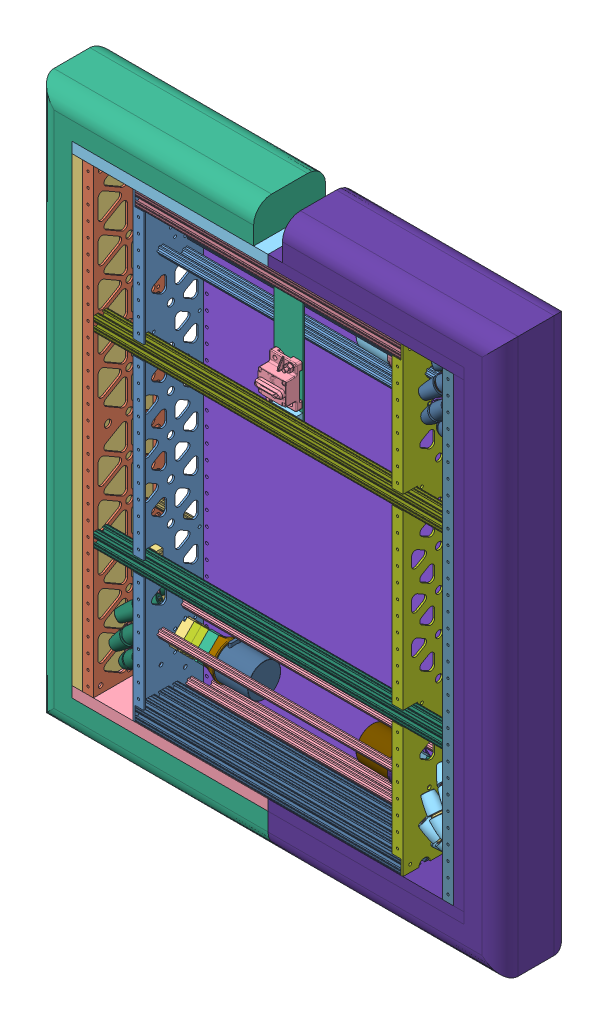
SolidWorks assembly Copy of Fame 2020, configuration Default. Lengths in mm. (continued)
Components (placement in the parent): (continued)
- Left Wheel Assembly v4(Mirror) (2)^Copy of Fame 2020-1: Left Wheel Assembly v4(Mirror) (2)^Copy of Fame 2020 [Default] at (500 0 0) x (1 0 0) z (0 0 -1) size (65.82 166.11 165.01) (virtual)
  - 6_Mecanum_Wheel_Left_217-2799 v1(Mirror) (2)^Left Wheel Assembly v4(Mirror) (2)_Copy of Fame 2020-1: 6_Mecanum_Wheel_Left_217-2799 v1(Mirror) (2)^Left Wheel Assembly v4(Mirror) (2)_Copy of Fame 2020 [Default] x (0 0 -1) z (1 0 0) size (165.01 166.11 65.82) (virtual)
    - 217-2799-001 Rev1(Mirror) (2)^6_Mecanum_Wheel_Left_217-2799 v1(Mirror) (2)_Left Wheel Assembly v4(Mirror) (2)_Copy of Fame 2020-1: 217-2799-001 Rev1(Mirror) (2)^6_Mecanum_Wheel_Left_217-2799 v1(Mirror) (2)_Left Wheel Assembly v4(Mirror) (2)_Copy of Fame 2020 [Default] at (33.3875 -317.5 -234.0098) x (0.707107 0.707107 0) z (0 0 1) size (95.78 100.46 28.55) (virtual)
    - 217-2799-001 Rev1(Mirror) (2)^6_Mecanum_Wheel_Left_217-2799 v1(Mirror) (2)_Left Wheel Assembly v4(Mirror) (2)_Copy of Fame 2020-2: 217-2799-001 Rev1(Mirror) (2)^6_Mecanum_Wheel_Left_217-2799 v1(Mirror) (2)_Left Wheel Assembly v4(Mirror) (2)_Copy of Fame 2020 [Default] at (33.3875 -317.5 -221.3098) x (-0.987688 -0.156434 0) z (0 0 -1) size (95.78 100.46 28.55) (virtual)
    - 217-2799-002 Rev1(Mirror) (2)^6_Mecanum_Wheel_Left_217-2799 v1(Mirror) (2)_Left Wheel Assembly v4(Mirror) (2)_Copy of Fame 2020-1: 217-2799-002 Rev1(Mirror) (2)^6_Mecanum_Wheel_Left_217-2799 v1(Mirror) (2)_Left Wheel Assembly v4(Mirror) (2)_Copy of Fame 2020 [Default] at (4.057 -346.8305 -227.6598) x (-0.707107 0.707107 0) z (0.707107 0.707107 0) size (26.84 25.39 30.1) (virtual)
    - 217-2799-002 Rev1(Mirror) (2)^6_Mecanum_Wheel_Left_217-2799 v1(Mirror) (2)_Left Wheel Assembly v4(Mirror) (2)_Copy of Fame 2020-2: 217-2799-002 Rev1(Mirror) (2)^6_Mecanum_Wheel_Left_217-2799 v1(Mirror) (2)_Left Wheel Assembly v4(Mirror) (2)_Copy of Fame 2020 [Default] at (-7.5815 -323.9888 -227.6598) x (-0.156434 0.987688 0) z (0.987688 0.156434 0) size (26.84 25.39 30.1) (virtual)
    - 217-2799-002 Rev1(Mirror) (2)^6_Mecanum_Wheel_Left_217-2799 v1(Mirror) (2)_Left Wheel Assembly v4(Mirror) (2)_Copy of Fame 2020-3: 217-2799-002 Rev1(Mirror) (2)^6_Mecanum_Wheel_Left_217-2799 v1(Mirror) (2)_Left Wheel Assembly v4(Mirror) (2)_Copy of Fame 2020 [Default] at (-3.5711 -298.6686 -227.6598) x (0.45399 0.891007 0) z (0.891007 -0.45399 0) size (26.84 25.39 30.1) (virtual)
    - 217-2799-002 Rev1(Mirror) (2)^6_Mecanum_Wheel_Left_217-2799 v1(Mirror) (2)_Left Wheel Assembly v4(Mirror) (2)_Copy of Fame 2020-4: 217-2799-002 Rev1(Mirror) (2)^6_Mecanum_Wheel_Left_217-2799 v1(Mirror) (2)_Left Wheel Assembly v4(Mirror) (2)_Copy of Fame 2020 [Default] at (14.5561 -280.5414 -227.6598) x (0.891007 0.45399 0) z (0.45399 -0.891007 0) size (26.84 25.39 30.1) (virtual)
    - 217-2799-002 Rev1(Mirror) (2)^6_Mecanum_Wheel_Left_217-2799 v1(Mirror) (2)_Left Wheel Assembly v4(Mirror) (2)_Copy of Fame 2020-5: 217-2799-002 Rev1(Mirror) (2)^6_Mecanum_Wheel_Left_217-2799 v1(Mirror) (2)_Left Wheel Assembly v4(Mirror) (2)_Copy of Fame 2020 [Default] at (39.8763 -276.531 -227.6598) x (0.987688 -0.156434 0) z (-0.156434 -0.987688 0) size (26.84 25.39 30.1) (virtual)
    - 217-2799-002 Rev1(Mirror) (2)^6_Mecanum_Wheel_Left_217-2799 v1(Mirror) (2)_Left Wheel Assembly v4(Mirror) (2)_Copy of Fame 2020-6: 217-2799-002 Rev1(Mirror) (2)^6_Mecanum_Wheel_Left_217-2799 v1(Mirror) (2)_Left Wheel Assembly v4(Mirror) (2)_Copy of Fame 2020 [Default] at (62.718 -288.1695 -227.6598) x (0.707107 -0.707107 0) z (-0.707107 -0.707107 0) size (26.84 25.39 30.1) (virtual)
    - 217-2799-002 Rev1(Mirror) (2)^6_Mecanum_Wheel_Left_217-2799 v1(Mirror) (2)_Left Wheel Assembly v4(Mirror) (2)_Copy of Fame 2020-7: 217-2799-002 Rev1(Mirror) (2)^6_Mecanum_Wheel_Left_217-2799 v1(Mirror) (2)_Left Wheel Assembly v4(Mirror) (2)_Copy of Fame 2020 [Default] at (74.3565 -311.0112 -227.6598) x (0.156434 -0.987688 0) z (-0.987688 -0.156434 0) size (26.84 25.39 30.1) (virtual)
    - 217-2799-002 Rev1(Mirror) (2)^6_Mecanum_Wheel_Left_217-2799 v1(Mirror) (2)_Left Wheel Assembly v4(Mirror) (2)_Copy of Fame 2020-8: 217-2799-002 Rev1(Mirror) (2)^6_Mecanum_Wheel_Left_217-2799 v1(Mirror) (2)_Left Wheel Assembly v4(Mirror) (2)_Copy of Fame 2020 [Default] at (70.3461 -336.3314 -227.6598) x (-0.45399 -0.891007 0) z (-0.891007 0.45399 0) size (26.84 25.39 30.1) (virtual)
    - 217-2799-002 Rev1(Mirror) (2)^6_Mecanum_Wheel_Left_217-2799 v1(Mirror) (2)_Left Wheel Assembly v4(Mirror) (2)_Copy of Fame 2020-9: 217-2799-002 Rev1(Mirror) (2)^6_Mecanum_Wheel_Left_217-2799 v1(Mirror) (2)_Left Wheel Assembly v4(Mirror) (2)_Copy of Fame 2020 [Default] at (52.2189 -354.4586 -227.6598) x (-0.891007 -0.45399 0) z (-0.45399 0.891007 0) size (26.84 25.39 30.1) (virtual)
    - 217-2799-002 Rev1(Mirror) (2)^6_Mecanum_Wheel_Left_217-2799 v1(Mirror) (2)_Left Wheel Assembly v4(Mirror) (2)_Copy of Fame 2020-10: 217-2799-002 Rev1(Mirror) (2)^6_Mecanum_Wheel_Left_217-2799 v1(Mirror) (2)_Left Wheel Assembly v4(Mirror) (2)_Copy of Fame 2020 [Default] at (26.8987 -358.469 -227.6598) x (-0.987688 0.156434 0) z (0.156434 0.987688 0) size (26.84 25.39 30.1) (virtual)
    - 217-2586-003 Rev2(Mirror) (2)^6_Mecanum_Wheel_Left_217-2799 v1(Mirror) (2)_Left Wheel Assembly v4(Mirror) (2)_Copy of Fame 2020-1: 217-2586-003 Rev2(Mirror) (2)^6_Mecanum_Wheel_Left_217-2799 v1(Mirror) (2)_Left Wheel Assembly v4(Mirror) (2)_Copy of Fame 2020 [Default] at (-13.4676 -358.6894 -223.6536) x (0.41944 0.854155 -0.30739) z (0.757674 -0.142894 0.636798) size (19.46 28.57 19.46) (virtual)
    - 217-2586-003 Rev2(Mirror) (2)^6_Mecanum_Wheel_Left_217-2799 v1(Mirror) (2)_Left Wheel Assembly v4(Mirror) (2)_Copy of Fame 2020-2: 217-2586-003 Rev2(Mirror) (2)^6_Mecanum_Wheel_Left_217-2799 v1(Mirror) (2)_Left Wheel Assembly v4(Mirror) (2)_Copy of Fame 2020 [Default] at (-7.8019 -364.3551 -231.666) x (0.847342 0.451134 0.280161) z (-0.17892 0.739241 -0.649238) size (19.46 28.57 19.46) (virtual)
    - 217-2586-003 Rev2(Mirror) (2)^6_Mecanum_Wheel_Left_217-2799 v1(Mirror) (2)_Left Wheel Assembly v4(Mirror) (2)_Copy of Fame 2020-3: 217-2586-003 Rev2(Mirror) (2)^6_Mecanum_Wheel_Left_217-2799 v1(Mirror) (2)_Left Wheel Assembly v4(Mirror) (2)_Copy of Fame 2020 [Default] at (-27.4761 -331.196 -231.666) x (0.950684 -0.13308 0.280161) z (0.289766 0.703225 -0.649238) size (19.46 28.57 19.46) (virtual)
    - 217-2586-003 Rev2(Mirror) (2)^6_Mecanum_Wheel_Left_217-2799 v1(Mirror) (2)_Left Wheel Assembly v4(Mirror) (2)_Copy of Fame 2020-4: 217-2586-003 Rev2(Mirror) (2)^6_Mecanum_Wheel_Left_217-2799 v1(Mirror) (2)_Left Wheel Assembly v4(Mirror) (2)_Copy of Fame 2020 [Default] at (-23.9025 -292.8056 -231.666) x (0.690897 -0.666462 0.280161) z (0.647771 0.398601 -0.649238) size (19.46 28.57 19.46) (virtual)
    - 217-2586-003 Rev2(Mirror) (2)^6_Mecanum_Wheel_Left_217-2799 v1(Mirror) (2)_Left Wheel Assembly v4(Mirror) (2)_Copy of Fame 2020-5: 217-2586-003 Rev2(Mirror) (2)^6_Mecanum_Wheel_Left_217-2799 v1(Mirror) (2)_Left Wheel Assembly v4(Mirror) (2)_Copy of Fame 2020 [Default] at (1.5539 -263.8475 -231.666) x (0.167211 -0.945278 0.280161) z (0.75835 -0.058276 -0.649238) size (19.46 28.57 19.46) (virtual)
    - 217-2586-003 Rev2(Mirror) (2)^6_Mecanum_Wheel_Left_217-2799 v1(Mirror) (2)_Left Wheel Assembly v4(Mirror) (2)_Copy of Fame 2020-6: 217-2586-003 Rev2(Mirror) (2)^6_Mecanum_Wheel_Left_217-2799 v1(Mirror) (2)_Left Wheel Assembly v4(Mirror) (2)_Copy of Fame 2020 [Default] at (39.1697 -255.3829 -231.666) x (-0.420344 -0.86303 0.280161) z (0.579264 -0.492893 -0.649238) size (19.46 28.57 19.46) (virtual)
    - 217-2586-003 Rev2(Mirror) (2)^6_Mecanum_Wheel_Left_217-2799 v1(Mirror) (2)_Left Wheel Assembly v4(Mirror) (2)_Copy of Fame 2020-7: 217-2586-003 Rev2(Mirror) (2)^6_Mecanum_Wheel_Left_217-2799 v1(Mirror) (2)_Left Wheel Assembly v4(Mirror) (2)_Copy of Fame 2020 [Default] at (74.5769 -270.6449 -231.666) x (-0.847342 -0.451134 0.280161) z (0.17892 -0.739241 -0.649238) size (19.46 28.57 19.46) (virtual)
    - 217-2586-003 Rev2(Mirror) (2)^6_Mecanum_Wheel_Left_217-2799 v1(Mirror) (2)_Left Wheel Assembly v4(Mirror) (2)_Copy of Fame 2020-8: 217-2586-003 Rev2(Mirror) (2)^6_Mecanum_Wheel_Left_217-2799 v1(Mirror) (2)_Left Wheel Assembly v4(Mirror) (2)_Copy of Fame 2020 [Default] at (94.2511 -303.804 -231.666) x (-0.950684 0.13308 0.280161) z (-0.289766 -0.703225 -0.649238) size (19.46 28.57 19.46) (virtual)
    - 217-2586-003 Rev2(Mirror) (2)^6_Mecanum_Wheel_Left_217-2799 v1(Mirror) (2)_Left Wheel Assembly v4(Mirror) (2)_Copy of Fame 2020-9: 217-2586-003 Rev2(Mirror) (2)^6_Mecanum_Wheel_Left_217-2799 v1(Mirror) (2)_Left Wheel Assembly v4(Mirror) (2)_Copy of Fame 2020 [Default] at (90.6775 -342.1944 -231.666) x (-0.690897 0.666462 0.280161) z (-0.647771 -0.398601 -0.649238) size (19.46 28.57 19.46) (virtual)
    - 217-2586-003 Rev2(Mirror) (2)^6_Mecanum_Wheel_Left_217-2799 v1(Mirror) (2)_Left Wheel Assembly v4(Mirror) (2)_Copy of Fame 2020-10: 217-2586-003 Rev2(Mirror) (2)^6_Mecanum_Wheel_Left_217-2799 v1(Mirror) (2)_Left Wheel Assembly v4(Mirror) (2)_Copy of Fame 2020 [Default] at (65.2211 -371.1525 -231.666) x (-0.167211 0.945278 0.280161) z (-0.75835 0.058276 -0.649238) size (19.46 28.57 19.46) (virtual)
    - 217-2586-003 Rev2(Mirror) (2)^6_Mecanum_Wheel_Left_217-2799 v1(Mirror) (2)_Left Wheel Assembly v4(Mirror) (2)_Copy of Fame 2020-11: 217-2586-003 Rev2(Mirror) (2)^6_Mecanum_Wheel_Left_217-2799 v1(Mirror) (2)_Left Wheel Assembly v4(Mirror) (2)_Copy of Fame 2020 [Default] at (27.6053 -379.6171 -231.666) x (0.420344 0.86303 0.280161) z (-0.579264 0.492893 -0.649238) size (19.46 28.57 19.46) (virtual)
    - 217-2586-003 Rev2(Mirror) (2)^6_Mecanum_Wheel_Left_217-2799 v1(Mirror) (2)_Left Wheel Assembly v4(Mirror) (2)_Copy of Fame 2020-12: 217-2586-003 Rev2(Mirror) (2)^6_Mecanum_Wheel_Left_217-2799 v1(Mirror) (2)_Left Wheel Assembly v4(Mirror) (2)_Copy of Fame 2020 [Default] at (-28.7296 -323.2822 -223.6536) x (0.841394 0.444485 -0.30739) z (0.52898 -0.560953 0.636798) size (19.46 28.57 19.46) (virtual)
    - 217-2586-003 Rev2(Mirror) (2)^6_Mecanum_Wheel_Left_217-2799 v1(Mirror) (2)_Left Wheel Assembly v4(Mirror) (2)_Copy of Fame 2020-13: 217-2586-003 Rev2(Mirror) (2)^6_Mecanum_Wheel_Left_217-2799 v1(Mirror) (2)_Left Wheel Assembly v4(Mirror) (2)_Copy of Fame 2020 [Default] at (-20.265 -285.6664 -223.6536) x (0.941964 -0.134963 -0.30739) z (0.098234 -0.764747 0.636798) size (19.46 28.57 19.46) (virtual)
    - 217-2586-003 Rev2(Mirror) (2)^6_Mecanum_Wheel_Left_217-2799 v1(Mirror) (2)_Left Wheel Assembly v4(Mirror) (2)_Copy of Fame 2020-14: 217-2586-003 Rev2(Mirror) (2)^6_Mecanum_Wheel_Left_217-2799 v1(Mirror) (2)_Left Wheel Assembly v4(Mirror) (2)_Copy of Fame 2020 [Default] at (8.6931 -260.21 -223.6536) x (0.682736 -0.66286 -0.30739) z (-0.370035 -0.676434 0.636798) size (19.46 28.57 19.46) (virtual)
    - 217-2586-003 Rev2(Mirror) (2)^6_Mecanum_Wheel_Left_217-2799 v1(Mirror) (2)_Left Wheel Assembly v4(Mirror) (2)_Copy of Fame 2020-15: 217-2586-003 Rev2(Mirror) (2)^6_Mecanum_Wheel_Left_217-2799 v1(Mirror) (2)_Left Wheel Assembly v4(Mirror) (2)_Copy of Fame 2020 [Default] at (47.0835 -256.6364 -223.6536) x (0.162726 -0.937567 -0.30739) z (-0.696962 -0.329746 0.636798) size (19.46 28.57 19.46) (virtual)
    - 217-2586-003 Rev2(Mirror) (2)^6_Mecanum_Wheel_Left_217-2799 v1(Mirror) (2)_Left Wheel Assembly v4(Mirror) (2)_Copy of Fame 2020-16: 217-2586-003 Rev2(Mirror) (2)^6_Mecanum_Wheel_Left_217-2799 v1(Mirror) (2)_Left Wheel Assembly v4(Mirror) (2)_Copy of Fame 2020 [Default] at (80.2426 -276.3106 -223.6536) x (-0.41944 -0.854155 -0.30739) z (-0.757674 0.142894 0.636798) size (19.46 28.57 19.46) (virtual)
    - 217-2586-003 Rev2(Mirror) (2)^6_Mecanum_Wheel_Left_217-2799 v1(Mirror) (2)_Left Wheel Assembly v4(Mirror) (2)_Copy of Fame 2020-17: 217-2586-003 Rev2(Mirror) (2)^6_Mecanum_Wheel_Left_217-2799 v1(Mirror) (2)_Left Wheel Assembly v4(Mirror) (2)_Copy of Fame 2020 [Default] at (95.5046 -311.7178 -223.6536) x (-0.841394 -0.444485 -0.30739) z (-0.52898 0.560953 0.636798) size (19.46 28.57 19.46) (virtual)
    - 217-2586-003 Rev2(Mirror) (2)^6_Mecanum_Wheel_Left_217-2799 v1(Mirror) (2)_Left Wheel Assembly v4(Mirror) (2)_Copy of Fame 2020-18: 217-2586-003 Rev2(Mirror) (2)^6_Mecanum_Wheel_Left_217-2799 v1(Mirror) (2)_Left Wheel Assembly v4(Mirror) (2)_Copy of Fame 2020 [Default] at (87.04 -349.3336 -223.6536) x (-0.941964 0.134963 -0.30739) z (-0.098234 0.764747 0.636798) size (19.46 28.57 19.46) (virtual)
    - 217-2586-003 Rev2(Mirror) (2)^6_Mecanum_Wheel_Left_217-2799 v1(Mirror) (2)_Left Wheel Assembly v4(Mirror) (2)_Copy of Fame 2020-19: 217-2586-003 Rev2(Mirror) (2)^6_Mecanum_Wheel_Left_217-2799 v1(Mirror) (2)_Left Wheel Assembly v4(Mirror) (2)_Copy of Fame 2020 [Default] at (58.0819 -374.79 -223.6536) x (-0.682736 0.66286 -0.30739) z (0.370035 0.676434 0.636798) size (19.46 28.57 19.46) (virtual)
    - 217-2586-003 Rev2(Mirror) (2)^6_Mecanum_Wheel_Left_217-2799 v1(Mirror) (2)_Left Wheel Assembly v4(Mirror) (2)_Copy of Fame 2020-20: 217-2586-003 Rev2(Mirror) (2)^6_Mecanum_Wheel_Left_217-2799 v1(Mirror) (2)_Left Wheel Assembly v4(Mirror) (2)_Copy of Fame 2020 [Default] at (19.6915 -378.3636 -223.6536) x (-0.162726 0.937567 -0.30739) z (0.696962 0.329746 0.636798) size (19.46 28.57 19.46) (virtual)
    - 217-2586-004 Rev1(Mirror) (2)^6_Mecanum_Wheel_Left_217-2799 v1(Mirror) (2)_Left Wheel Assembly v4(Mirror) (2)_Copy of Fame 2020-1: 217-2586-004 Rev1(Mirror) (2)^6_Mecanum_Wheel_Left_217-2799 v1(Mirror) (2)_Left Wheel Assembly v4(Mirror) (2)_Copy of Fame 2020 [Default] at (-10.3479 -361.809 -228.0654) x (-0.690521 -0.722949 0.02293) z (-0.522667 0.476807 -0.706735) size (25.9 28.58 25.9) (virtual)
    - 217-2586-004 Rev1(Mirror) (2)^6_Mecanum_Wheel_Left_217-2799 v1(Mirror) (2)_Left Wheel Assembly v4(Mirror) (2)_Copy of Fame 2020-2: 217-2586-004 Rev1(Mirror) (2)^6_Mecanum_Wheel_Left_217-2799 v1(Mirror) (2)_Left Wheel Assembly v4(Mirror) (2)_Copy of Fame 2020 [Default] at (-10.9209 -361.2361 -227.2551) x (0.01458 -0.811521 0.584142) z (0.865903 0.302381 0.39847) size (25.9 28.58 25.9) (virtual)
    - 217-2586-004 Rev1(Mirror) (2)^6_Mecanum_Wheel_Left_217-2799 v1(Mirror) (2)_Left Wheel Assembly v4(Mirror) (2)_Copy of Fame 2020-3: 217-2586-004 Rev1(Mirror) (2)^6_Mecanum_Wheel_Left_217-2799 v1(Mirror) (2)_Left Wheel Assembly v4(Mirror) (2)_Copy of Fame 2020 [Default] at (-28.1662 -326.8394 -227.2551) x (-0.465204 -0.665104 0.584142) z (0.878265 -0.264334 0.39847) size (25.9 28.58 25.9) (virtual)
    - 217-2586-004 Rev1(Mirror) (2)^6_Mecanum_Wheel_Left_217-2799 v1(Mirror) (2)_Left Wheel Assembly v4(Mirror) (2)_Copy of Fame 2020-4: 217-2586-004 Rev1(Mirror) (2)^6_Mecanum_Wheel_Left_217-2799 v1(Mirror) (2)_Left Wheel Assembly v4(Mirror) (2)_Copy of Fame 2020 [Default] at (-21.9 -288.8754 -227.2551) x (-0.767297 -0.26464 0.584142) z (0.55516 -0.730082 0.39847) size (25.9 28.58 25.9) (virtual)
    - 217-2586-004 Rev1(Mirror) (2)^6_Mecanum_Wheel_Left_217-2799 v1(Mirror) (2)_Left Wheel Assembly v4(Mirror) (2)_Copy of Fame 2020-5: 217-2586-004 Rev1(Mirror) (2)^6_Mecanum_Wheel_Left_217-2799 v1(Mirror) (2)_Left Wheel Assembly v4(Mirror) (2)_Copy of Fame 2020 [Default] at (5.484 -261.845 -227.2551) x (-0.776308 0.236907 0.584142) z (0.020002 -0.916963 0.39847) size (25.9 28.58 25.9) (virtual)
    - 217-2586-004 Rev1(Mirror) (2)^6_Mecanum_Wheel_Left_217-2799 v1(Mirror) (2)_Left Wheel Assembly v4(Mirror) (2)_Copy of Fame 2020-6: 217-2586-004 Rev1(Mirror) (2)^6_Mecanum_Wheel_Left_217-2799 v1(Mirror) (2)_Left Wheel Assembly v4(Mirror) (2)_Copy of Fame 2020 [Default] at (43.5263 -256.0729 -227.2551) x (-0.488796 0.647964 0.584142) z (-0.522795 -0.753596 0.39847) size (25.9 28.58 25.9) (virtual)
    - 217-2586-004 Rev1(Mirror) (2)^6_Mecanum_Wheel_Left_217-2799 v1(Mirror) (2)_Left Wheel Assembly v4(Mirror) (2)_Copy of Fame 2020-7: 217-2586-004 Rev1(Mirror) (2)^6_Mecanum_Wheel_Left_217-2799 v1(Mirror) (2)_Left Wheel Assembly v4(Mirror) (2)_Copy of Fame 2020 [Default] at (77.6959 -273.7639 -227.2551) x (-0.01458 0.811521 0.584142) z (-0.865903 -0.302381 0.39847) size (25.9 28.58 25.9) (virtual)
    - 217-2586-004 Rev1(Mirror) (2)^6_Mecanum_Wheel_Left_217-2799 v1(Mirror) (2)_Left Wheel Assembly v4(Mirror) (2)_Copy of Fame 2020-8: 217-2586-004 Rev1(Mirror) (2)^6_Mecanum_Wheel_Left_217-2799 v1(Mirror) (2)_Left Wheel Assembly v4(Mirror) (2)_Copy of Fame 2020 [Default] at (94.9412 -308.1606 -227.2551) x (0.465204 0.665104 0.584142) z (-0.878265 0.264334 0.39847) size (25.9 28.58 25.9) (virtual)
    - 217-2586-004 Rev1(Mirror) (2)^6_Mecanum_Wheel_Left_217-2799 v1(Mirror) (2)_Left Wheel Assembly v4(Mirror) (2)_Copy of Fame 2020-9: 217-2586-004 Rev1(Mirror) (2)^6_Mecanum_Wheel_Left_217-2799 v1(Mirror) (2)_Left Wheel Assembly v4(Mirror) (2)_Copy of Fame 2020 [Default] at (88.675 -346.1246 -227.2551) x (0.767297 0.26464 0.584142) z (-0.55516 0.730082 0.39847) size (25.9 28.58 25.9) (virtual)
    - 217-2586-004 Rev1(Mirror) (2)^6_Mecanum_Wheel_Left_217-2799 v1(Mirror) (2)_Left Wheel Assembly v4(Mirror) (2)_Copy of Fame 2020-10: 217-2586-004 Rev1(Mirror) (2)^6_Mecanum_Wheel_Left_217-2799 v1(Mirror) (2)_Left Wheel Assembly v4(Mirror) (2)_Copy of Fame 2020 [Default] at (61.291 -373.155 -227.2551) x (0.776308 -0.236907 0.584142) z (-0.020002 0.916963 0.39847) size (25.9 28.58 25.9) (virtual)
    - 217-2586-004 Rev1(Mirror) (2)^6_Mecanum_Wheel_Left_217-2799 v1(Mirror) (2)_Left Wheel Assembly v4(Mirror) (2)_Copy of Fame 2020-11: 217-2586-004 Rev1(Mirror) (2)^6_Mecanum_Wheel_Left_217-2799 v1(Mirror) (2)_Left Wheel Assembly v4(Mirror) (2)_Copy of Fame 2020 [Default] at (23.2487 -378.9271 -227.2551) x (0.488796 -0.647964 0.584142) z (0.522795 0.753596 0.39847) size (25.9 28.58 25.9) (virtual)
    - 217-2586-004 Rev1(Mirror) (2)^6_Mecanum_Wheel_Left_217-2799 v1(Mirror) (2)_Left Wheel Assembly v4(Mirror) (2)_Copy of Fame 2020-12: 217-2586-004 Rev1(Mirror) (2)^6_Mecanum_Wheel_Left_217-2799 v1(Mirror) (2)_Left Wheel Assembly v4(Mirror) (2)_Copy of Fame 2020 [Default] at (-28.0394 -327.6397 -228.0654) x (-0.983582 -0.179 0.02293) z (-0.142587 0.692961 -0.706735) size (25.9 28.58 25.9) (virtual)
    - 217-2586-004 Rev1(Mirror) (2)^6_Mecanum_Wheel_Left_217-2799 v1(Mirror) (2)_Left Wheel Assembly v4(Mirror) (2)_Copy of Fame 2020-13: 217-2586-004 Rev1(Mirror) (2)^6_Mecanum_Wheel_Left_217-2799 v1(Mirror) (2)_Left Wheel Assembly v4(Mirror) (2)_Copy of Fame 2020 [Default] at (-22.2679 -289.5974 -228.0654) x (-0.900948 0.433321 0.02293) z (0.291957 0.644427 -0.706735) size (25.9 28.58 25.9) (virtual)
    - 217-2586-004 Rev1(Mirror) (2)^6_Mecanum_Wheel_Left_217-2799 v1(Mirror) (2)_Left Wheel Assembly v4(Mirror) (2)_Copy of Fame 2020-14: 217-2586-004 Rev1(Mirror) (2)^6_Mecanum_Wheel_Left_217-2799 v1(Mirror) (2)_Left Wheel Assembly v4(Mirror) (2)_Copy of Fame 2020 [Default] at (4.7621 -262.2129 -228.0654) x (-0.474183 0.880128 0.02293) z (0.614983 0.349745 -0.706735) size (25.9 28.58 25.9) (virtual)
    - 217-2586-004 Rev1(Mirror) (2)^6_Mecanum_Wheel_Left_217-2799 v1(Mirror) (2)_Left Wheel Assembly v4(Mirror) (2)_Copy of Fame 2020-15: 217-2586-004 Rev1(Mirror) (2)^6_Mecanum_Wheel_Left_217-2799 v1(Mirror) (2)_Left Wheel Assembly v4(Mirror) (2)_Copy of Fame 2020 [Default] at (42.726 -255.9462 -228.0654) x (0.133704 0.990756 0.02293) z (0.703107 -0.078529 -0.706735) size (25.9 28.58 25.9) (virtual)
    - 217-2586-004 Rev1(Mirror) (2)^6_Mecanum_Wheel_Left_217-2799 v1(Mirror) (2)_Left Wheel Assembly v4(Mirror) (2)_Copy of Fame 2020-16: 217-2586-004 Rev1(Mirror) (2)^6_Mecanum_Wheel_Left_217-2799 v1(Mirror) (2)_Left Wheel Assembly v4(Mirror) (2)_Copy of Fame 2020 [Default] at (77.1229 -273.191 -228.0654) x (0.690521 0.722949 0.02293) z (0.522667 -0.476807 -0.706735) size (25.9 28.58 25.9) (virtual)
    - 217-2586-004 Rev1(Mirror) (2)^6_Mecanum_Wheel_Left_217-2799 v1(Mirror) (2)_Left Wheel Assembly v4(Mirror) (2)_Copy of Fame 2020-17: 217-2586-004 Rev1(Mirror) (2)^6_Mecanum_Wheel_Left_217-2799 v1(Mirror) (2)_Left Wheel Assembly v4(Mirror) (2)_Copy of Fame 2020 [Default] at (94.8144 -307.3603 -228.0654) x (0.983582 0.179 0.02293) z (0.142587 -0.692961 -0.706735) size (25.9 28.58 25.9) (virtual)
    - 217-2586-004 Rev1(Mirror) (2)^6_Mecanum_Wheel_Left_217-2799 v1(Mirror) (2)_Left Wheel Assembly v4(Mirror) (2)_Copy of Fame 2020-18: 217-2586-004 Rev1(Mirror) (2)^6_Mecanum_Wheel_Left_217-2799 v1(Mirror) (2)_Left Wheel Assembly v4(Mirror) (2)_Copy of Fame 2020 [Default] at (89.0429 -345.4026 -228.0654) x (0.900948 -0.433321 0.02293) z (-0.291957 -0.644427 -0.706735) size (25.9 28.58 25.9) (virtual)
    - 217-2586-004 Rev1(Mirror) (2)^6_Mecanum_Wheel_Left_217-2799 v1(Mirror) (2)_Left Wheel Assembly v4(Mirror) (2)_Copy of Fame 2020-19: 217-2586-004 Rev1(Mirror) (2)^6_Mecanum_Wheel_Left_217-2799 v1(Mirror) (2)_Left Wheel Assembly v4(Mirror) (2)_Copy of Fame 2020 [Default] at (62.0129 -372.7871 -228.0654) x (0.474183 -0.880128 0.02293) z (-0.614983 -0.349745 -0.706735) size (25.9 28.58 25.9) (virtual)
    - 217-2586-004 Rev1(Mirror) (2)^6_Mecanum_Wheel_Left_217-2799 v1(Mirror) (2)_Left Wheel Assembly v4(Mirror) (2)_Copy of Fame 2020-20: 217-2586-004 Rev1(Mirror) (2)^6_Mecanum_Wheel_Left_217-2799 v1(Mirror) (2)_Left Wheel Assembly v4(Mirror) (2)_Copy of Fame 2020 [Default] at (24.049 -379.0538 -228.0654) x (-0.133704 -0.990756 0.02293) z (-0.703107 0.078529 -0.706735) size (25.9 28.58 25.9) (virtual)
    - 217-2586-007 Rev1(Mirror) (2)^6_Mecanum_Wheel_Left_217-2799 v1(Mirror) (2)_Left Wheel Assembly v4(Mirror) (2)_Copy of Fame 2020-1: 217-2586-007 Rev1(Mirror) (2)^6_Mecanum_Wheel_Left_217-2799 v1(Mirror) (2)_Left Wheel Assembly v4(Mirror) (2)_Copy of Fame 2020 [Default] at (-10.6347 -361.5222 -227.6598) x (0.5 -0.5 -0.707107) z (0.709055 0.705148 0.002763) size (61.72 5 5) (virtual)
    - 217-2586-007 Rev1(Mirror) (2)^6_Mecanum_Wheel_Left_217-2799 v1(Mirror) (2)_Left Wheel Assembly v4(Mirror) (2)_Copy of Fame 2020-2: 217-2586-007 Rev1(Mirror) (2)^6_Mecanum_Wheel_Left_217-2799 v1(Mirror) (2)_Left Wheel Assembly v4(Mirror) (2)_Copy of Fame 2020 [Default] at (-28.1029 -327.2391 -227.6598) x (0.110616 -0.698401 -0.707107) z (0.988113 0.153705 0.002763) size (61.72 5 5) (virtual)
    - 217-2586-007 Rev1(Mirror) (2)^6_Mecanum_Wheel_Left_217-2799 v1(Mirror) (2)_Left Wheel Assembly v4(Mirror) (2)_Copy of Fame 2020-3: 217-2586-007 Rev1(Mirror) (2)^6_Mecanum_Wheel_Left_217-2799 v1(Mirror) (2)_Left Wheel Assembly v4(Mirror) (2)_Copy of Fame 2020 [Default] at (-22.0838 -289.236 -227.6598) x (-0.32102 -0.630037 -0.707107) z (0.889746 -0.456448 0.002763) size (61.72 5 5) (virtual)
    - 217-2586-007 Rev1(Mirror) (2)^6_Mecanum_Wheel_Left_217-2799 v1(Mirror) (2)_Left Wheel Assembly v4(Mirror) (2)_Copy of Fame 2020-4: 217-2586-007 Rev1(Mirror) (2)^6_Mecanum_Wheel_Left_217-2799 v1(Mirror) (2)_Left Wheel Assembly v4(Mirror) (2)_Copy of Fame 2020 [Default] at (5.1235 -262.0287 -227.6598) x (-0.630037 -0.32102 -0.707107) z (0.451526 -0.892254 0.002763) size (61.72 5 5) (virtual)
    - 217-2586-007 Rev1(Mirror) (2)^6_Mecanum_Wheel_Left_217-2799 v1(Mirror) (2)_Left Wheel Assembly v4(Mirror) (2)_Copy of Fame 2020-5: 217-2586-007 Rev1(Mirror) (2)^6_Mecanum_Wheel_Left_217-2799 v1(Mirror) (2)_Left Wheel Assembly v4(Mirror) (2)_Copy of Fame 2020 [Default] at (43.1266 -256.0096 -227.6598) x (-0.698401 0.110616 -0.707107) z (-0.159162 -0.987249 0.002763) size (61.72 5 5) (virtual)
    - 217-2586-007 Rev1(Mirror) (2)^6_Mecanum_Wheel_Left_217-2799 v1(Mirror) (2)_Left Wheel Assembly v4(Mirror) (2)_Copy of Fame 2020-6: 217-2586-007 Rev1(Mirror) (2)^6_Mecanum_Wheel_Left_217-2799 v1(Mirror) (2)_Left Wheel Assembly v4(Mirror) (2)_Copy of Fame 2020 [Default] at (77.4097 -273.4778 -227.6598) x (-0.5 0.5 -0.707107) z (-0.709055 -0.705148 0.002763) size (61.72 5 5) (virtual)
    - 217-2586-007 Rev1(Mirror) (2)^6_Mecanum_Wheel_Left_217-2799 v1(Mirror) (2)_Left Wheel Assembly v4(Mirror) (2)_Copy of Fame 2020-7: 217-2586-007 Rev1(Mirror) (2)^6_Mecanum_Wheel_Left_217-2799 v1(Mirror) (2)_Left Wheel Assembly v4(Mirror) (2)_Copy of Fame 2020 [Default] at (94.8779 -307.7609 -227.6598) x (-0.110616 0.698401 -0.707107) z (-0.988113 -0.153705 0.002763) size (61.72 5 5) (virtual)
    - 217-2586-007 Rev1(Mirror) (2)^6_Mecanum_Wheel_Left_217-2799 v1(Mirror) (2)_Left Wheel Assembly v4(Mirror) (2)_Copy of Fame 2020-8: 217-2586-007 Rev1(Mirror) (2)^6_Mecanum_Wheel_Left_217-2799 v1(Mirror) (2)_Left Wheel Assembly v4(Mirror) (2)_Copy of Fame 2020 [Default] at (88.8588 -345.764 -227.6598) x (0.32102 0.630037 -0.707107) z (-0.889746 0.456448 0.002763) size (61.72 5 5) (virtual)
    - 217-2586-007 Rev1(Mirror) (2)^6_Mecanum_Wheel_Left_217-2799 v1(Mirror) (2)_Left Wheel Assembly v4(Mirror) (2)_Copy of Fame 2020-9: 217-2586-007 Rev1(Mirror) (2)^6_Mecanum_Wheel_Left_217-2799 v1(Mirror) (2)_Left Wheel Assembly v4(Mirror) (2)_Copy of Fame 2020 [Default] at (61.6515 -372.9713 -227.6598) x (0.630037 0.32102 -0.707107) z (-0.451526 0.892254 0.002763) size (61.72 5 5) (virtual)
    - 217-2586-007 Rev1(Mirror) (2)^6_Mecanum_Wheel_Left_217-2799 v1(Mirror) (2)_Left Wheel Assembly v4(Mirror) (2)_Copy of Fame 2020-10: 217-2586-007 Rev1(Mirror) (2)^6_Mecanum_Wheel_Left_217-2799 v1(Mirror) (2)_Left Wheel Assembly v4(Mirror) (2)_Copy of Fame 2020 [Default] at (23.6484 -378.9904 -227.6598) x (0.698401 -0.110616 -0.707107) z (0.159162 0.987249 0.002763) size (61.72 5 5) (virtual)
    - 217-2586-008 Rev1(Mirror) (2)^6_Mecanum_Wheel_Left_217-2799 v1(Mirror) (2)_Left Wheel Assembly v4(Mirror) (2)_Copy of Fame 2020-1: 217-2586-008 Rev1(Mirror) (2)^6_Mecanum_Wheel_Left_217-2799 v1(Mirror) (2)_Left Wheel Assembly v4(Mirror) (2)_Copy of Fame 2020 [Default] at (53.3583 -330.4692 -227.5328) x (0.544639 0.838671 0) z (0 0 -1) size (7.33 6.35 31.75) (virtual)
    - 217-2586-008 Rev1(Mirror) (2)^6_Mecanum_Wheel_Left_217-2799 v1(Mirror) (2)_Left Wheel Assembly v4(Mirror) (2)_Copy of Fame 2020-2: 217-2586-008 Rev1(Mirror) (2)^6_Mecanum_Wheel_Left_217-2799 v1(Mirror) (2)_Left Wheel Assembly v4(Mirror) (2)_Copy of Fame 2020 [Default] at (32.1413 -341.2799 -227.5328) x (0.99863 -0.052336 0) z (0 0 -1) size (7.33 6.35 31.75) (virtual)
    - 217-2586-008 Rev1(Mirror) (2)^6_Mecanum_Wheel_Left_217-2799 v1(Mirror) (2)_Left Wheel Assembly v4(Mirror) (2)_Copy of Fame 2020-3: 217-2586-008 Rev1(Mirror) (2)^6_Mecanum_Wheel_Left_217-2799 v1(Mirror) (2)_Left Wheel Assembly v4(Mirror) (2)_Copy of Fame 2020 [Default] at (12.1704 -328.3106 -227.5328) x (0.45399 -0.891007 0) z (0 0 -1) size (7.33 6.35 31.75) (virtual)
    - 217-2586-008 Rev1(Mirror) (2)^6_Mecanum_Wheel_Left_217-2799 v1(Mirror) (2)_Left Wheel Assembly v4(Mirror) (2)_Copy of Fame 2020-4: 217-2586-008 Rev1(Mirror) (2)^6_Mecanum_Wheel_Left_217-2799 v1(Mirror) (2)_Left Wheel Assembly v4(Mirror) (2)_Copy of Fame 2020 [Default] at (13.4167 -304.5308 -227.5328) x (-0.544639 -0.838671 0) z (0 0 -1) size (7.33 6.35 31.75) (virtual)
    - 217-2586-008 Rev1(Mirror) (2)^6_Mecanum_Wheel_Left_217-2799 v1(Mirror) (2)_Left Wheel Assembly v4(Mirror) (2)_Copy of Fame 2020-5: 217-2586-008 Rev1(Mirror) (2)^6_Mecanum_Wheel_Left_217-2799 v1(Mirror) (2)_Left Wheel Assembly v4(Mirror) (2)_Copy of Fame 2020 [Default] at (34.6337 -293.7201 -227.5328) x (-0.99863 0.052336 0) z (0 0 -1) size (7.33 6.35 31.75) (virtual)
    - 217-2586-008 Rev1(Mirror) (2)^6_Mecanum_Wheel_Left_217-2799 v1(Mirror) (2)_Left Wheel Assembly v4(Mirror) (2)_Copy of Fame 2020-6: 217-2586-008 Rev1(Mirror) (2)^6_Mecanum_Wheel_Left_217-2799 v1(Mirror) (2)_Left Wheel Assembly v4(Mirror) (2)_Copy of Fame 2020 [Default] at (54.6046 -306.6894 -227.5328) x (-0.45399 0.891007 0) z (0 0 -1) size (7.33 6.35 31.75) (virtual)
    - NUT-832-NYLOCK(Mirror) (2)^6_Mecanum_Wheel_Left_217-2799 v1(Mirror) (2)_Left Wheel Assembly v4(Mirror) (2)_Copy of Fame 2020-1: NUT-832-NYLOCK(Mirror) (2)^6_Mecanum_Wheel_Left_217-2799 v1(Mirror) (2)_Left Wheel Assembly v4(Mirror) (2)_Copy of Fame 2020 [Default] at (6.1639 -290.2764 -241.3161) x (0.258819 -0.965926 0) z (0.965926 0.258819 0) size (9.37 5.86 8.12) (virtual)
    - NUT-832-NYLOCK(Mirror) (2)^6_Mecanum_Wheel_Left_217-2799 v1(Mirror) (2)_Left Wheel Assembly v4(Mirror) (2)_Copy of Fame 2020-2: NUT-832-NYLOCK(Mirror) (2)^6_Mecanum_Wheel_Left_217-2799 v1(Mirror) (2)_Left Wheel Assembly v4(Mirror) (2)_Copy of Fame 2020 [Default] at (-0.9163 -334.9786 -241.3161) x (0.99863 -0.052336 0) z (0.052336 0.99863 0) size (9.37 5.86 8.12) (virtual)
    - NUT-832-NYLOCK(Mirror) (2)^6_Mecanum_Wheel_Left_217-2799 v1(Mirror) (2)_Left Wheel Assembly v4(Mirror) (2)_Copy of Fame 2020-3: NUT-832-NYLOCK(Mirror) (2)^6_Mecanum_Wheel_Left_217-2799 v1(Mirror) (2)_Left Wheel Assembly v4(Mirror) (2)_Copy of Fame 2020 [Default] at (39.4102 -355.526 -241.3161) x (0.358368 0.93358 0) z (-0.93358 0.358368 0) size (9.37 5.86 8.12) (virtual)
    - NUT-832-NYLOCK(Mirror) (2)^6_Mecanum_Wheel_Left_217-2799 v1(Mirror) (2)_Left Wheel Assembly v4(Mirror) (2)_Copy of Fame 2020-4: NUT-832-NYLOCK(Mirror) (2)^6_Mecanum_Wheel_Left_217-2799 v1(Mirror) (2)_Left Wheel Assembly v4(Mirror) (2)_Copy of Fame 2020 [Default] at (71.4135 -323.5227 -241.3161) x (-0.777146 0.62932 0) z (-0.62932 -0.777146 0) size (9.37 5.86 8.12) (virtual)
    - NUT-832-NYLOCK(Mirror) (2)^6_Mecanum_Wheel_Left_217-2799 v1(Mirror) (2)_Left Wheel Assembly v4(Mirror) (2)_Copy of Fame 2020-5: NUT-832-NYLOCK(Mirror) (2)^6_Mecanum_Wheel_Left_217-2799 v1(Mirror) (2)_Left Wheel Assembly v4(Mirror) (2)_Copy of Fame 2020 [Default] at (50.8661 -283.1962 -241.3161) x (-0.838671 -0.544639 0) z (0.544639 -0.838671 0) size (9.37 5.86 8.12) (virtual)
    - SCREW-832-1250(Mirror) (2)^6_Mecanum_Wheel_Left_217-2799 v1(Mirror) (2)_Left Wheel Assembly v4(Mirror) (2)_Copy of Fame 2020-1: SCREW-832-1250(Mirror) (2)^6_Mecanum_Wheel_Left_217-2799 v1(Mirror) (2)_Left Wheel Assembly v4(Mirror) (2)_Copy of Fame 2020 [Default] at (6.1639 -290.2764 -212.75) x (0 0 -1) z (0.394243 -0.919006 0) size (33.96 7.92 7.92) (virtual)
    - SCREW-832-1250(Mirror) (2)^6_Mecanum_Wheel_Left_217-2799 v1(Mirror) (2)_Left Wheel Assembly v4(Mirror) (2)_Copy of Fame 2020-2: SCREW-832-1250(Mirror) (2)^6_Mecanum_Wheel_Left_217-2799 v1(Mirror) (2)_Left Wheel Assembly v4(Mirror) (2)_Copy of Fame 2020 [Default] at (-0.9163 -334.9786 -212.75) x (0 0 -1) z (0.995855 0.090959 0) size (33.96 7.92 7.92) (virtual)
    - SCREW-832-1250(Mirror) (2)^6_Mecanum_Wheel_Left_217-2799 v1(Mirror) (2)_Left Wheel Assembly v4(Mirror) (2)_Copy of Fame 2020-3: SCREW-832-1250(Mirror) (2)^6_Mecanum_Wheel_Left_217-2799 v1(Mirror) (2)_Left Wheel Assembly v4(Mirror) (2)_Copy of Fame 2020 [Default] at (39.4102 -355.526 -212.75) x (0 0 -1) z (0.221229 0.975222 0) size (33.96 7.92 7.92) (virtual)
    - SCREW-832-1250(Mirror) (2)^6_Mecanum_Wheel_Left_217-2799 v1(Mirror) (2)_Left Wheel Assembly v4(Mirror) (2)_Copy of Fame 2020-4: SCREW-832-1250(Mirror) (2)^6_Mecanum_Wheel_Left_217-2799 v1(Mirror) (2)_Left Wheel Assembly v4(Mirror) (2)_Copy of Fame 2020 [Default] at (71.4135 -323.5227 -212.75) x (0 0 -1) z (-0.859128 0.511761 0) size (33.96 7.92 7.92) (virtual)
    - SCREW-832-1250(Mirror) (2)^6_Mecanum_Wheel_Left_217-2799 v1(Mirror) (2)_Left Wheel Assembly v4(Mirror) (2)_Copy of Fame 2020-5: SCREW-832-1250(Mirror) (2)^6_Mecanum_Wheel_Left_217-2799 v1(Mirror) (2)_Left Wheel Assembly v4(Mirror) (2)_Copy of Fame 2020 [Default] at (50.8661 -283.1962 -212.75) x (0 0 -1) z (-0.752199 -0.658936 0) size (33.96 7.92 7.92) (virtual)
    - 217-2586-005 Rev2(Mirror) (2)^6_Mecanum_Wheel_Left_217-2799 v1(Mirror) (2)_Left Wheel Assembly v4(Mirror) (2)_Copy of Fame 2020-1: 217-2586-005 Rev2(Mirror) (2)^6_Mecanum_Wheel_Left_217-2799 v1(Mirror) (2)_Left Wheel Assembly v4(Mirror) (2)_Copy of Fame 2020 [Default] at (-6.1597 -365.9972 -233.9884) x (-0.5 0.5 0.707107) z (-0.146447 -0.853553 0.5) size (8.5 8 8) (virtual)
    - 217-2586-005 Rev2(Mirror) (2)^6_Mecanum_Wheel_Left_217-2799 v1(Mirror) (2)_Left Wheel Assembly v4(Mirror) (2)_Copy of Fame 2020-2: 217-2586-005 Rev2(Mirror) (2)^6_Mecanum_Wheel_Left_217-2799 v1(Mirror) (2)_Left Wheel Assembly v4(Mirror) (2)_Copy of Fame 2020 [Default] at (-15.1097 -357.0472 -221.3312) x (-0.5 0.5 0.707107) z (-0.146447 -0.853553 0.5) size (8.5 8 8) (virtual)
    - 217-2586-005 Rev2(Mirror) (2)^6_Mecanum_Wheel_Left_217-2799 v1(Mirror) (2)_Left Wheel Assembly v4(Mirror) (2)_Copy of Fame 2020-3: 217-2586-005 Rev2(Mirror) (2)^6_Mecanum_Wheel_Left_217-2799 v1(Mirror) (2)_Left Wheel Assembly v4(Mirror) (2)_Copy of Fame 2020 [Default] at (-29.0929 -320.9884 -221.3312) x (-0.110616 0.698401 0.707107) z (-0.620184 -0.60446 0.5) size (8.5 8 8) (virtual)
    - 217-2586-005 Rev2(Mirror) (2)^6_Mecanum_Wheel_Left_217-2799 v1(Mirror) (2)_Left Wheel Assembly v4(Mirror) (2)_Copy of Fame 2020-4: 217-2586-005 Rev2(Mirror) (2)^6_Mecanum_Wheel_Left_217-2799 v1(Mirror) (2)_Left Wheel Assembly v4(Mirror) (2)_Copy of Fame 2020 [Default] at (-19.2106 -283.5972 -221.3312) x (0.32102 0.630037 0.707107) z (-0.857032 -0.124484 0.5) size (8.5 8 8) (virtual)
    - 217-2586-005 Rev2(Mirror) (2)^6_Mecanum_Wheel_Left_217-2799 v1(Mirror) (2)_Left Wheel Assembly v4(Mirror) (2)_Copy of Fame 2020-5: 217-2586-005 Rev2(Mirror) (2)^6_Mecanum_Wheel_Left_217-2799 v1(Mirror) (2)_Left Wheel Assembly v4(Mirror) (2)_Copy of Fame 2020 [Default] at (10.7623 -259.1556 -221.3312) x (0.630037 0.32102 0.707107) z (-0.766523 0.403042 0.5) size (8.5 8 8) (virtual)
    - 217-2586-005 Rev2(Mirror) (2)^6_Mecanum_Wheel_Left_217-2799 v1(Mirror) (2)_Left Wheel Assembly v4(Mirror) (2)_Copy of Fame 2020-6: 217-2586-005 Rev2(Mirror) (2)^6_Mecanum_Wheel_Left_217-2799 v1(Mirror) (2)_Left Wheel Assembly v4(Mirror) (2)_Copy of Fame 2020 [Default] at (49.3773 -256.9997 -221.3312) x (0.698401 -0.110616 0.707107) z (-0.383228 0.776618 0.5) size (8.5 8 8) (virtual)
    - 217-2586-005 Rev2(Mirror) (2)^6_Mecanum_Wheel_Left_217-2799 v1(Mirror) (2)_Left Wheel Assembly v4(Mirror) (2)_Copy of Fame 2020-7: 217-2586-005 Rev2(Mirror) (2)^6_Mecanum_Wheel_Left_217-2799 v1(Mirror) (2)_Left Wheel Assembly v4(Mirror) (2)_Copy of Fame 2020 [Default] at (81.8847 -277.9528 -221.3312) x (0.5 -0.5 0.707107) z (0.146447 0.853553 0.5) size (8.5 8 8) (virtual)
    - 217-2586-005 Rev2(Mirror) (2)^6_Mecanum_Wheel_Left_217-2799 v1(Mirror) (2)_Left Wheel Assembly v4(Mirror) (2)_Copy of Fame 2020-8: 217-2586-005 Rev2(Mirror) (2)^6_Mecanum_Wheel_Left_217-2799 v1(Mirror) (2)_Left Wheel Assembly v4(Mirror) (2)_Copy of Fame 2020 [Default] at (95.8679 -314.0116 -221.3312) x (0.110616 -0.698401 0.707107) z (0.620184 0.60446 0.5) size (8.5 8 8) (virtual)
    - 217-2586-005 Rev2(Mirror) (2)^6_Mecanum_Wheel_Left_217-2799 v1(Mirror) (2)_Left Wheel Assembly v4(Mirror) (2)_Copy of Fame 2020-9: 217-2586-005 Rev2(Mirror) (2)^6_Mecanum_Wheel_Left_217-2799 v1(Mirror) (2)_Left Wheel Assembly v4(Mirror) (2)_Copy of Fame 2020 [Default] at (85.9856 -351.4028 -221.3312) x (-0.32102 -0.630037 0.707107) z (0.857032 0.124484 0.5) size (8.5 8 8) (virtual)
    - 217-2586-005 Rev2(Mirror) (2)^6_Mecanum_Wheel_Left_217-2799 v1(Mirror) (2)_Left Wheel Assembly v4(Mirror) (2)_Copy of Fame 2020-10: 217-2586-005 Rev2(Mirror) (2)^6_Mecanum_Wheel_Left_217-2799 v1(Mirror) (2)_Left Wheel Assembly v4(Mirror) (2)_Copy of Fame 2020 [Default] at (56.0127 -375.8444 -221.3312) x (-0.630037 -0.32102 0.707107) z (0.766523 -0.403042 0.5) size (8.5 8 8) (virtual)
    - 217-2586-005 Rev2(Mirror) (2)^6_Mecanum_Wheel_Left_217-2799 v1(Mirror) (2)_Left Wheel Assembly v4(Mirror) (2)_Copy of Fame 2020-11: 217-2586-005 Rev2(Mirror) (2)^6_Mecanum_Wheel_Left_217-2799 v1(Mirror) (2)_Left Wheel Assembly v4(Mirror) (2)_Copy of Fame 2020 [Default] at (17.3977 -378.0003 -221.3312) x (-0.698401 0.110616 0.707107) z (0.383228 -0.776618 0.5) size (8.5 8 8) (virtual)
    - 217-2586-005 Rev2(Mirror) (2)^6_Mecanum_Wheel_Left_217-2799 v1(Mirror) (2)_Left Wheel Assembly v4(Mirror) (2)_Copy of Fame 2020-12: 217-2586-005 Rev2(Mirror) (2)^6_Mecanum_Wheel_Left_217-2799 v1(Mirror) (2)_Left Wheel Assembly v4(Mirror) (2)_Copy of Fame 2020 [Default] at (-27.1128 -333.4898 -233.9884) x (-0.110616 0.698401 0.707107) z (-0.620184 -0.60446 0.5) size (8.5 8 8) (virtual)
    - 217-2586-005 Rev2(Mirror) (2)^6_Mecanum_Wheel_Left_217-2799 v1(Mirror) (2)_Left Wheel Assembly v4(Mirror) (2)_Copy of Fame 2020-13: 217-2586-005 Rev2(Mirror) (2)^6_Mecanum_Wheel_Left_217-2799 v1(Mirror) (2)_Left Wheel Assembly v4(Mirror) (2)_Copy of Fame 2020 [Default] at (-24.9569 -294.8748 -233.9884) x (0.32102 0.630037 0.707107) z (-0.857032 -0.124484 0.5) size (8.5 8 8) (virtual)
    - 217-2586-005 Rev2(Mirror) (2)^6_Mecanum_Wheel_Left_217-2799 v1(Mirror) (2)_Left Wheel Assembly v4(Mirror) (2)_Copy of Fame 2020-14: 217-2586-005 Rev2(Mirror) (2)^6_Mecanum_Wheel_Left_217-2799 v1(Mirror) (2)_Left Wheel Assembly v4(Mirror) (2)_Copy of Fame 2020 [Default] at (-0.5153 -264.9019 -233.9884) x (0.630037 0.32102 0.707107) z (-0.766523 0.403042 0.5) size (8.5 8 8) (virtual)
    - 217-2586-005 Rev2(Mirror) (2)^6_Mecanum_Wheel_Left_217-2799 v1(Mirror) (2)_Left Wheel Assembly v4(Mirror) (2)_Copy of Fame 2020-15: 217-2586-005 Rev2(Mirror) (2)^6_Mecanum_Wheel_Left_217-2799 v1(Mirror) (2)_Left Wheel Assembly v4(Mirror) (2)_Copy of Fame 2020 [Default] at (36.8759 -255.0196 -233.9884) x (0.698401 -0.110616 0.707107) z (-0.383228 0.776618 0.5) size (8.5 8 8) (virtual)
    - 217-2586-005 Rev2(Mirror) (2)^6_Mecanum_Wheel_Left_217-2799 v1(Mirror) (2)_Left Wheel Assembly v4(Mirror) (2)_Copy of Fame 2020-16: 217-2586-005 Rev2(Mirror) (2)^6_Mecanum_Wheel_Left_217-2799 v1(Mirror) (2)_Left Wheel Assembly v4(Mirror) (2)_Copy of Fame 2020 [Default] at (72.9347 -269.0028 -233.9884) x (0.5 -0.5 0.707107) z (0.146447 0.853553 0.5) size (8.5 8 8) (virtual)
    - 217-2586-005 Rev2(Mirror) (2)^6_Mecanum_Wheel_Left_217-2799 v1(Mirror) (2)_Left Wheel Assembly v4(Mirror) (2)_Copy of Fame 2020-17: 217-2586-005 Rev2(Mirror) (2)^6_Mecanum_Wheel_Left_217-2799 v1(Mirror) (2)_Left Wheel Assembly v4(Mirror) (2)_Copy of Fame 2020 [Default] at (93.8878 -301.5102 -233.9884) x (0.110616 -0.698401 0.707107) z (0.620184 0.60446 0.5) size (8.5 8 8) (virtual)
    - 217-2586-005 Rev2(Mirror) (2)^6_Mecanum_Wheel_Left_217-2799 v1(Mirror) (2)_Left Wheel Assembly v4(Mirror) (2)_Copy of Fame 2020-18: 217-2586-005 Rev2(Mirror) (2)^6_Mecanum_Wheel_Left_217-2799 v1(Mirror) (2)_Left Wheel Assembly v4(Mirror) (2)_Copy of Fame 2020 [Default] at (91.7319 -340.1252 -233.9884) x (-0.32102 -0.630037 0.707107) z (0.857032 0.124484 0.5) size (8.5 8 8) (virtual)
    - 217-2586-005 Rev2(Mirror) (2)^6_Mecanum_Wheel_Left_217-2799 v1(Mirror) (2)_Left Wheel Assembly v4(Mirror) (2)_Copy of Fame 2020-19: 217-2586-005 Rev2(Mirror) (2)^6_Mecanum_Wheel_Left_217-2799 v1(Mirror) (2)_Left Wheel Assembly v4(Mirror) (2)_Copy of Fame 2020 [Default] at (67.2903 -370.0981 -233.9884) x (-0.630037 -0.32102 0.707107) z (0.766523 -0.403042 0.5) size (8.5 8 8) (virtual)
    - 217-2586-005 Rev2(Mirror) (2)^6_Mecanum_Wheel_Left_217-2799 v1(Mirror) (2)_Left Wheel Assembly v4(Mirror) (2)_Copy of Fame 2020-20: 217-2586-005 Rev2(Mirror) (2)^6_Mecanum_Wheel_Left_217-2799 v1(Mirror) (2)_Left Wheel Assembly v4(Mirror) (2)_Copy of Fame 2020 [Default] at (29.8991 -379.9804 -233.9884) x (-0.698401 0.110616 0.707107) z (0.383228 -0.776618 0.5) size (8.5 8 8) (virtual)
  - 1_2_Hex_Bore_Aluminum_VersaHub_217-2592 v1(Mirror) (2)^Left Wheel Assembly v4(Mirror) (2)_Copy of Fame 2020-1: 1_2_Hex_Bore_Aluminum_VersaHub_217-2592 v1(Mirror) (2)^Left Wheel Assembly v4(Mirror) (2)_Copy of Fame 2020 [Default] at (-239.7248 -317.5 -33.3875) x (-1 0 0) z (0 -0.707107 0.707107) size (12.7 55.88 55.88) (virtual)
- NEO Gearbox 2-stage Custom v5(Mirror)^Copy of Fame 2020-1: NEO Gearbox 2-stage Custom v5(Mirror)^Copy of Fame 2020 [Default] at (0 0 425) x (-1 0 0) z (0 0 -1) size (164.9 90.53 90.53) (virtual)
  - VersaPlanetary_4_1_Gear_Kit_217-2818 v1(Mirror)^NEO Gearbox 2-stage Custom v5(Mirror)_Copy of Fame 2020-1: VersaPlanetary_4_1_Gear_Kit_217-2818 v1(Mirror)^NEO Gearbox 2-stage Custom v5(Mirror)_Copy of Fame 2020 [Default] at (-15.25 22.225 0) x (0 -0.707107 -0.707107) z (1 0 0) size (35.49 35.49 17.4) (virtual)
    - 217-2725-001 Rev1_24t Sun(Mirror)^VersaPlanetary_4_1_Gear_Kit_217-2818 v1(Mirror)_NEO Gearbox 2-stage Custom v5(Mirror)_Copy of Fame 2020-1: 217-2725-001 Rev1_24t Sun(Mirror)^VersaPlanetary_4_1_Gear_Kit_217-2818 v1(Mirror)_NEO Gearbox 2-stage Custom v5(Mirror)_Copy of Fame 2020 [Default] at (-36.69 -517.1337 209.675) x (0.707107 0.707107 0) z (0 0 1) size (14.4 14.45 12.7) (virtual)
    - 217-2725-002 Rev1_24t Planet(Mirror)^VersaPlanetary_4_1_Gear_Kit_217-2818 v1(Mirror)_NEO Gearbox 2-stage Custom v5(Mirror)_Copy of Fame 2020-1: 217-2725-002 Rev1_24t Planet(Mirror)^VersaPlanetary_4_1_Gear_Kit_217-2818 v1(Mirror)_NEO Gearbox 2-stage Custom v5(Mirror)_Copy of Fame 2020 [Default] at (-45.2382 -525.6819 212.025) x (-0.793353 0.608761 0) z (0 0 -1) size (13.12 13.1 8) (virtual)
    - 217-2725-002 Rev1_24t Planet(Mirror)^VersaPlanetary_4_1_Gear_Kit_217-2818 v1(Mirror)_NEO Gearbox 2-stage Custom v5(Mirror)_Copy of Fame 2020-2: 217-2725-002 Rev1_24t Planet(Mirror)^VersaPlanetary_4_1_Gear_Kit_217-2818 v1(Mirror)_NEO Gearbox 2-stage Custom v5(Mirror)_Copy of Fame 2020 [Default] at (-28.1418 -525.6819 212.025) x (-0.608761 -0.793353 0) z (0 0 -1) size (13.12 13.1 8) (virtual)
    - 217-2725-002 Rev1_24t Planet(Mirror)^VersaPlanetary_4_1_Gear_Kit_217-2818 v1(Mirror)_NEO Gearbox 2-stage Custom v5(Mirror)_Copy of Fame 2020-3: 217-2725-002 Rev1_24t Planet(Mirror)^VersaPlanetary_4_1_Gear_Kit_217-2818 v1(Mirror)_NEO Gearbox 2-stage Custom v5(Mirror)_Copy of Fame 2020 [Default] at (-28.1418 -508.5855 212.025) x (0.793353 -0.608761 0) z (0 0 -1) size (13.12 13.1 8) (virtual)
    - 217-2725-002 Rev1_24t Planet(Mirror)^VersaPlanetary_4_1_Gear_Kit_217-2818 v1(Mirror)_NEO Gearbox 2-stage Custom v5(Mirror)_Copy of Fame 2020-4: 217-2725-002 Rev1_24t Planet(Mirror)^VersaPlanetary_4_1_Gear_Kit_217-2818 v1(Mirror)_NEO Gearbox 2-stage Custom v5(Mirror)_Copy of Fame 2020 [Default] at (-45.2382 -508.5855 212.025) x (0.608761 0.793353 0) z (0 0 -1) size (13.12 13.1 8) (virtual)
    - 217-2724-002 Rev1(Mirror)^VersaPlanetary_4_1_Gear_Kit_217-2818 v1(Mirror)_NEO Gearbox 2-stage Custom v5(Mirror)_Copy of Fame 2020-1: 217-2724-002 Rev1(Mirror)^VersaPlanetary_4_1_Gear_Kit_217-2818 v1(Mirror)_NEO Gearbox 2-stage Custom v5(Mirror)_Copy of Fame 2020 [Default] at (-36.69 -517.1337 218.375) x (1 0 0) z (0 0 -1) size (34.7 34.7 4.7) (virtual)
    - 217-2625-010 Rev1(Mirror)^VersaPlanetary_4_1_Gear_Kit_217-2818 v1(Mirror)_NEO Gearbox 2-stage Custom v5(Mirror)_Copy of Fame 2020-1: 217-2625-010 Rev1(Mirror)^VersaPlanetary_4_1_Gear_Kit_217-2818 v1(Mirror)_NEO Gearbox 2-stage Custom v5(Mirror)_Copy of Fame 2020 [Default] at (-45.2382 -525.6819 214.725) x (0.854322 0.519745 0) z (0 0 1) size (4 4 12) (virtual)
    - 217-2625-010 Rev1(Mirror)^VersaPlanetary_4_1_Gear_Kit_217-2818 v1(Mirror)_NEO Gearbox 2-stage Custom v5(Mirror)_Copy of Fame 2020-2: 217-2625-010 Rev1(Mirror)^VersaPlanetary_4_1_Gear_Kit_217-2818 v1(Mirror)_NEO Gearbox 2-stage Custom v5(Mirror)_Copy of Fame 2020 [Default] at (-28.1418 -525.6819 214.725) x (-0.519745 0.854322 0) z (0 0 1) size (4 4 12) (virtual)
    - 217-2625-010 Rev1(Mirror)^VersaPlanetary_4_1_Gear_Kit_217-2818 v1(Mirror)_NEO Gearbox 2-stage Custom v5(Mirror)_Copy of Fame 2020-3: 217-2625-010 Rev1(Mirror)^VersaPlanetary_4_1_Gear_Kit_217-2818 v1(Mirror)_NEO Gearbox 2-stage Custom v5(Mirror)_Copy of Fame 2020 [Default] at (-28.1418 -508.5855 214.725) x (-0.854322 -0.519745 0) z (0 0 1) size (4 4 12) (virtual)
    - 217-2625-010 Rev1(Mirror)^VersaPlanetary_4_1_Gear_Kit_217-2818 v1(Mirror)_NEO Gearbox 2-stage Custom v5(Mirror)_Copy of Fame 2020-4: 217-2625-010 Rev1(Mirror)^VersaPlanetary_4_1_Gear_Kit_217-2818 v1(Mirror)_NEO Gearbox 2-stage Custom v5(Mirror)_Copy of Fame 2020 [Default] at (-45.2382 -508.5855 214.725) x (0.519745 -0.854322 0) z (0 0 1) size (4 4 12) (virtual)
  - 217-2625-026 Rev1(Mirror)^NEO Gearbox 2-stage Custom v5(Mirror)_Copy of Fame 2020-1: 217-2625-026 Rev1(Mirror)^NEO Gearbox 2-stage Custom v5(Mirror)_Copy of Fame 2020 [Default] at (211.875 -317.5 391.6125) x (0 -0.707107 -0.707107) z (1 0 0) size (44.45 42 18.12) (virtual)
  - 217-2742-001 Rev4(Mirror)^NEO Gearbox 2-stage Custom v5(Mirror)_Copy of Fame 2020-1: 217-2742-001 Rev4(Mirror)^NEO Gearbox 2-stage Custom v5(Mirror)_Copy of Fame 2020 [Default] at (218.5752 -317.5 391.6125) x (1 0 0) z (0 -0.63857 0.769564) size (7 28 28) (virtual)
  - 217-2742-001 Rev4(Mirror)^NEO Gearbox 2-stage Custom v5(Mirror)_Copy of Fame 2020-2: 217-2742-001 Rev4(Mirror)^NEO Gearbox 2-stage Custom v5(Mirror)_Copy of Fame 2020 [Default] at (226.5752 -317.5 391.6125) x (1 0 0) z (0 -0.707107 0.707107) size (7 28 28) (virtual)
  - 217-2625-017 Rev1_9714K61(Mirror)^NEO Gearbox 2-stage Custom v5(Mirror)_Copy of Fame 2020-1: 217-2625-017 Rev1_9714K61(Mirror)^NEO Gearbox 2-stage Custom v5(Mirror)_Copy of Fame 2020 [Default] at (225.795 -317.6887 391.9075) x (0 0.983393 -0.181491) z (0 0.181491 0.983393) size (28.51 4.98 27.43) (virtual)
  - 217-2625-025 Rev1(Mirror)^NEO Gearbox 2-stage Custom v5(Mirror)_Copy of Fame 2020-1: 217-2625-025 Rev1(Mirror)^NEO Gearbox 2-stage Custom v5(Mirror)_Copy of Fame 2020 [Default] at (182.475 -317.5 391.6125) x (0 -0.707107 -0.707107) z (1 0 0) size (44.45 42 18) (virtual)
  - 217-2816-001 Rev1(Mirror)^NEO Gearbox 2-stage Custom v5(Mirror)_Copy of Fame 2020-1: 217-2816-001 Rev1(Mirror)^NEO Gearbox 2-stage Custom v5(Mirror)_Copy of Fame 2020 [Default] at (212.025 -317.5 391.6125) x (0 -0.707107 -0.707107) z (-1 0 0) size (42 42 14.5) (virtual)
  - 217-2816-001 Rev1(Mirror)^NEO Gearbox 2-stage Custom v5(Mirror)_Copy of Fame 2020-2: 217-2816-001 Rev1(Mirror)^NEO Gearbox 2-stage Custom v5(Mirror)_Copy of Fame 2020 [Default] at (199.325 -317.5 391.6125) x (0 -0.707107 -0.707107) z (-1 0 0) size (42 42 14.5) (virtual)
  - 217-4649-001 Rev1(Mirror)^NEO Gearbox 2-stage Custom v5(Mirror)_Copy of Fame 2020-1: 217-4649-001 Rev1(Mirror)^NEO Gearbox 2-stage Custom v5(Mirror)_Copy of Fame 2020 [Default] at (185.629 -317.5 391.6125) x (0 -0.707107 -0.707107) z (-1 0 0) size (18 18 13) (virtual)
  - VersaPlanetary_CIM_Adapter_217-4018 v1(Mirror)^NEO Gearbox 2-stage Custom v5(Mirror)_Copy of Fame 2020-1: VersaPlanetary_CIM_Adapter_217-4018 v1(Mirror)^NEO Gearbox 2-stage Custom v5(Mirror)_Copy of Fame 2020 [Default] at (165.15 -317.5 391.6125) x (0 -0.707107 -0.707107) z (0 -0.707107 0.707107) size (64.01 21.55 64.01) (virtual)
  - NEO Motor REV-21-1650 v2(Mirror)^NEO Gearbox 2-stage Custom v5(Mirror)_Copy of Fame 2020-1: NEO Motor REV-21-1650 v2(Mirror)^NEO Gearbox 2-stage Custom v5(Mirror)_Copy of Fame 2020 [Default] at (153.625 -317.5 391.6125) x (0 -0.707107 0.707107) z (-1 0 0) size (61.14 61.02 93.25) (virtual)
  - 3_1 Output Shaft Custom v6(Mirror)^NEO Gearbox 2-stage Custom v5(Mirror)_Copy of Fame 2020-1: 3_1 Output Shaft Custom v6(Mirror)^NEO Gearbox 2-stage Custom v5(Mirror)_Copy of Fame 2020 [Default] at (211.3752 -317.5 391.6125) x (1 0 0) z (0 -0.707107 0.707107) size (48.9 34.7 34.7) (virtual)
